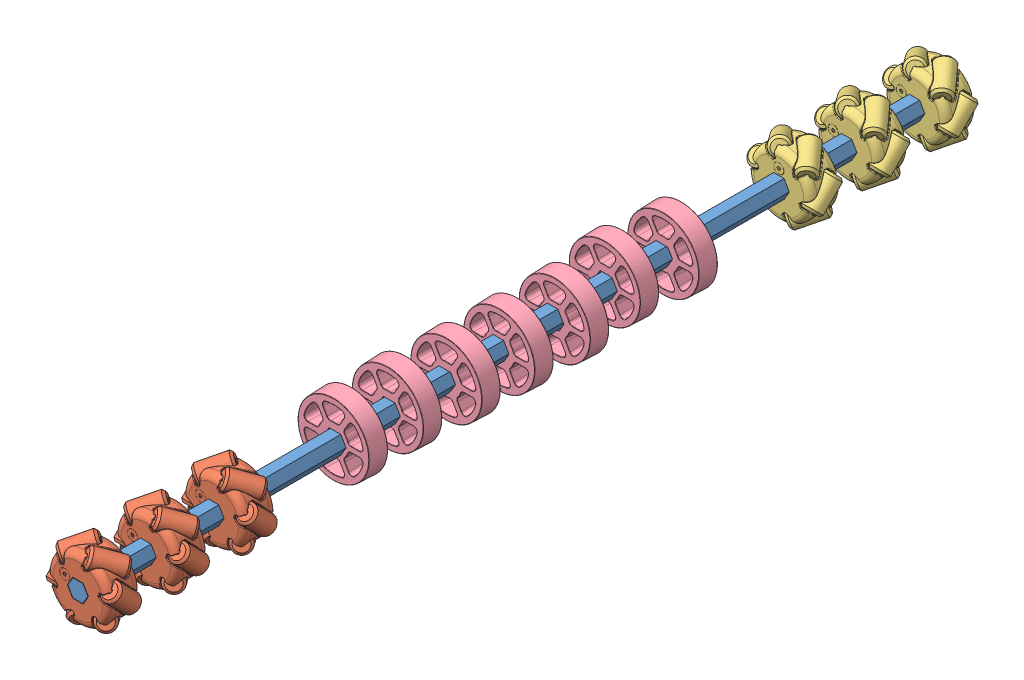
SolidWorks assembly mech intake, configuration Default. Lengths in mm.
Overall size (70.21 69.88 611.73).
14 component instances, 4 part files, 41 mates.
Components (placement in the parent):
- Hex shaft 0.5-1: Hex shaft 0.5 [Default] at (18.4614 91.3272 95.7371) size (14.66 12.7 609.6)
- TTB-0010-RH-1: TTB-0010-RH [Default] at (18.5054 91.3272 116.3746) x (-0.866025 0.5 0) z (0.5 0.866025 0) size (51.61 24.36 50.8)
- TTB-0010-RH-2: TTB-0010-RH [Default] at (18.5054 91.3272 163.9996) x (-0.866025 0.5 0) z (0.5 0.866025 0) size (51.61 24.36 50.8)
- TTB-0010-RH-3: TTB-0010-RH [Default] at (18.4834 91.3653 211.6246) x (-0.866025 0.5 0) z (0.5 0.866025 0) size (51.61 24.36 50.8)
- TTB-0010-LH-1: TTB-0010-LH [Default] at (18.5274 91.3653 -280.5004) x (0 -1 0) z (-1 0 0) size (51.61 24.36 50.8)
- TTB-0010-LH-2: TTB-0010-LH [Default] at (18.4834 91.3653 -375.7504) x (0.866025 -0.5 0) z (-0.5 -0.866025 0) size (51.61 24.36 50.8)
- TTB-0010-LH-3: TTB-0010-LH [Default] at (18.3954 91.2891 -328.1254) x (0.866025 -0.5 0) z (-0.5 -0.866025 0) size (51.61 24.36 50.8)
- 2in compliant wheel-1: 2in compliant wheel [Default] at (19.8179 90.3747 -123.3379) size (50.78 50.78 12.71)
- 2in compliant wheel-2: 2in compliant wheel [Default] at (19.9645 92.0257 -47.1379) size (50.78 50.78 12.71)
- 2in compliant wheel-3: 2in compliant wheel [Default] at (19.0113 90.3747 -85.2379) size (50.78 50.78 12.71)
- 2in compliant wheel-4: 2in compliant wheel [Default] at (16.9583 92.0257 29.0621) size (50.78 50.78 12.71)
- 2in compliant wheel-5: 2in compliant wheel [Default] at (19.9645 92.0257 -199.5379) size (50.78 50.78 12.71)
- 2in compliant wheel-7: 2in compliant wheel [Default] at (16.8116 92.2797 -161.4379) size (50.78 50.78 12.71)
- 2in compliant wheel-9: 2in compliant wheel [Default] at (16.9583 92.0257 -9.0379) size (50.78 50.78 12.71)
Mates (geometry in assembly coordinates):
- Coincident1: coincident anti-aligned: plane of Hex shaft 0.5-1 through (14.7952 97.6772 -386.8629) normal (-0.866025 0.5 0); plane of TTB-0010-RH-1 through (14.8172 97.7153 127.4871) normal (0.866025 -0.5 0)
- Coincident2: coincident anti-aligned: plane of Hex shaft 0.5-1 through (11.129 91.3272 -386.8629) normal (-0.866025 -0.5 0); plane of TTB-0010-RH-1 through (11.129 91.3272 127.4871) normal (0.866025 0.5 0)
- Coincident3: coincident anti-aligned: plane of Hex shaft 0.5-1 through (11.129 91.3272 -386.8629) normal (-0.866025 -0.5 0); plane of TTB-0010-RH-2 through (11.129 91.3272 175.1121) normal (0.866025 0.5 0)
- Coincident4: coincident anti-aligned: plane of Hex shaft 0.5-1 through (14.7952 97.6772 -386.8629) normal (-0.866025 0.5 0); plane of TTB-0010-RH-2 through (14.8172 97.7153 175.1121) normal (0.866025 -0.5 0)
- Coincident5: coincident anti-aligned: plane of Hex shaft 0.5-1 through (11.129 91.3272 -386.8629) normal (-0.866025 -0.5 0); plane of TTB-0010-RH-3 through (11.107 91.3653 222.7371) normal (0.866025 0.5 0)
- Coincident7: coincident anti-aligned: plane of Hex shaft 0.5-1 through (11.129 91.3272 -386.8629) normal (-0.866025 -0.5 0); plane of TTB-0010-RH-3 through (11.107 91.3653 222.7371) normal (0.866025 0.5 0)
- Coincident8: coincident anti-aligned: plane of Hex shaft 0.5-1 through (14.7952 84.9772 -386.8629) normal (0 -1 0); plane of TTB-0010-RH-3 through (14.7952 84.9772 222.7371) normal (0 1 0)
- Coincident9: coincident anti-aligned: plane of Hex shaft 0.5-1 through (14.7952 84.9772 -386.8629) normal (0 -1 0); plane of TTB-0010-LH-2 through (22.1716 84.9772 -364.6379) normal (0 1 0)
- Parallel1: parallel anti-aligned: plane of Hex shaft 0.5-1 through (22.1276 97.6772 -386.8629) normal (0 1 0); plane of TTB-0010-LH-2 through (14.7952 97.7534 -364.6379) normal (0 -1 0)
- Coincident11: coincident anti-aligned: plane of Hex shaft 0.5-1 through (11.129 91.3272 -386.8629) normal (-0.866025 -0.5 0); plane of TTB-0010-LH-2 through (14.7952 84.9772 -364.6379) normal (0.866025 0.5 0)
- Coincident12: coincident anti-aligned: plane of Hex shaft 0.5-1 through (14.7952 84.9772 -386.8629) normal (0 -1 0); plane of TTB-0010-LH-1 through (22.2156 84.9772 -269.3879) normal (0 1 0)
- Coincident13: coincident anti-aligned: plane of Hex shaft 0.5-1 through (14.7952 97.6772 -386.8629) normal (-0.866025 0.5 0); plane of TTB-0010-LH-1 through (11.151 91.3653 -269.3879) normal (0.866025 -0.5 0)
- Coincident15: coincident anti-aligned: plane of Hex shaft 0.5-1 through (22.1276 84.9772 -386.8629) normal (0.866025 -0.5 0); plane of TTB-0010-LH-3 through (25.7717 91.2891 -317.0129) normal (-0.866025 0.5 0)
- Coincident17: coincident anti-aligned: plane of Hex shaft 0.5-1 through (22.1276 97.6772 -386.8629) normal (0 1 0); plane of TTB-0010-LH-3 through (14.7072 97.6772 -317.0129) normal (0 -1 0)
- Coincident22: coincident aligned: plane of Hex shaft 0.5-1 through (18.4614 91.3272 -386.8629) normal (0 0 -1); plane of TTB-0010-LH-2 through (18.4834 91.3653 -386.8629) normal (0 0 -1)
- Distance2: distance = 25.4 mm anti-aligned: plane of TTB-0010-LH-2 through (18.4834 91.3653 -364.6379) normal (0 0 1); plane of TTB-0010-LH-3 through (18.3954 91.2891 -339.2379) normal (0 0 -1)
- Distance3: distance = 25.4 mm: plane of TTB-0010-LH-1 through (18.5274 91.3653 -291.6129) normal (0 0 -1); point of TTB-0010-LH-3
- Coincident29: coincident aligned: plane of Hex shaft 0.5-1 through (18.4614 91.3272 222.7371) normal (0 0 1); plane of TTB-0010-RH-3 through (18.4834 91.3653 222.7371) normal (0 0 1)
- Distance5: distance = 25.4 mm anti-aligned: plane of TTB-0010-RH-2 through (18.5054 91.3272 175.1121) normal (0 0 1); plane of TTB-0010-RH-3 through (18.4834 91.3653 200.5121) normal (0 0 -1)
- Distance6: distance = 25.4 mm anti-aligned: plane of TTB-0010-RH-2 through (18.5054 91.3272 152.8871) normal (0 0 -1); plane of TTB-0010-RH-1 through (18.5054 91.3272 127.4871) normal (0 0 1)
- Coincident32: coincident anti-aligned: plane of Hex shaft 0.5-1 through (22.1276 84.9772 -386.8629) normal (0.866025 -0.5 0); plane of 2in compliant wheel-2 through (26.197 92.0257 -34.436) normal (-0.866025 0.5 0)
- Coincident33: coincident: plane of Hex shaft 0.5-1 through (22.1276 97.6772 -386.8629) normal (0 1 0); line of 2in compliant wheel-2 through (23.2274 97.6772 -47.1379) axis (-1 0 0)
- Coincident34: coincident anti-aligned: plane of Hex shaft 0.5-1 through (14.7952 84.9772 -386.8629) normal (0 -1 0); plane of 2in compliant wheel-3 through (22.1276 84.9772 -72.536) normal (0 1 0)
- Parallel2: parallel anti-aligned: plane of Hex shaft 0.5-1 through (22.1276 97.6772 -386.8629) normal (0 1 0); plane of 2in compliant wheel-3 through (15.8951 95.7722 -72.536) normal (0 -1 0)
- Coincident36: coincident anti-aligned: plane of Hex shaft 0.5-1 through (22.1276 84.9772 -386.8629) normal (0.866025 -0.5 0); plane of 2in compliant wheel-3 through (25.2438 90.3747 -72.536) normal (-0.866025 0.5 0)
- Coincident37: coincident anti-aligned: plane of Hex shaft 0.5-1 through (22.1276 97.6772 -386.8629) normal (0 1 0); plane of 2in compliant wheel-7 through (13.6954 97.6772 -148.736) normal (0 -1 0)
- Coincident41: coincident: plane of Hex shaft 0.5-1 through (22.1276 97.6772 -386.8629) normal (0 1 0); line of 2in compliant wheel-9 through (20.2212 97.6772 -9.0379) axis (-1 0 0)
- Coincident42: coincident anti-aligned: plane of Hex shaft 0.5-1 through (11.129 91.3272 -386.8629) normal (-0.866025 -0.5 0); plane of 2in compliant wheel-9 through (13.842 86.6282 3.664) normal (0.866025 0.5 0)
- Coincident43: coincident: plane of Hex shaft 0.5-1 through (22.1276 97.6772 -386.8629) normal (0 1 0); line of 2in compliant wheel-4 through (20.2212 97.6772 29.0621) axis (-1 0 0)
- Coincident44: coincident anti-aligned: plane of Hex shaft 0.5-1 through (11.129 91.3272 -386.8629) normal (-0.866025 -0.5 0); plane of 2in compliant wheel-4 through (13.842 86.6282 41.764) normal (0.866025 0.5 0)
- Distance9: distance = 25.4 mm anti-aligned: plane of 2in compliant wheel-4 through (16.9583 92.0257 29.0621) normal (0 0 -1); plane of 2in compliant wheel-9 through (16.9583 92.0257 3.6621) normal (0 0 1)
- Distance10: distance = 25.4 mm anti-aligned: plane of 2in compliant wheel-2 through (19.9645 92.0257 -34.4379) normal (0 0 1); plane of 2in compliant wheel-9 through (16.9583 92.0257 -9.0379) normal (0 0 -1)
- Distance11: distance = 25.4 mm anti-aligned: plane of 2in compliant wheel-3 through (19.0113 90.3747 -72.5379) normal (0 0 1); plane of 2in compliant wheel-2 through (19.9645 92.0257 -47.1379) normal (0 0 -1)
- Coincident50: coincident anti-aligned: plane of Hex shaft 0.5-1 through (14.7952 84.9772 -386.8629) normal (0 -1 0); plane of 2in compliant wheel-1 through (22.9341 84.9772 -110.636) normal (0 1 0)
- Coincident52: coincident: plane of Hex shaft 0.5-1 through (25.7937 91.3272 -386.8629) normal (0.866025 0.5 0); line of 2in compliant wheel-1 through (23.0808 96.0262 -110.6379) axis (0.5 -0.866025 0)
- Distance12: distance = 25.4 mm anti-aligned: plane of 2in compliant wheel-1 through (19.8179 90.3747 -110.6379) normal (0 0 1); plane of 2in compliant wheel-3 through (19.0113 90.3747 -85.2379) normal (0 0 -1)
- Coincident55: coincident: plane of Hex shaft 0.5-1 through (22.1276 97.6772 -386.8629) normal (0 1 0); line of 2in compliant wheel-5 through (16.7016 97.6772 -186.8379) axis (1 0 0)
- Coincident56: coincident anti-aligned: plane of Hex shaft 0.5-1 through (22.1276 84.9772 -386.8629) normal (0.866025 -0.5 0); plane of 2in compliant wheel-5 through (26.197 92.0257 -186.836) normal (-0.866025 0.5 0)
- Distance13: distance = 25.4 mm anti-aligned: plane of 2in compliant wheel-5 through (19.9645 92.0257 -186.8379) normal (0 0 1); plane of 2in compliant wheel-7 through (16.8116 92.2797 -161.4379) normal (0 0 -1)
- Distance14: distance = 25.4 mm anti-aligned: plane of 2in compliant wheel-7 through (16.8116 92.2797 -148.7379) normal (0 0 1); plane of 2in compliant wheel-1 through (19.8179 90.3747 -123.3379) normal (0 0 -1)
- Coincident59: coincident anti-aligned: plane of Hex shaft 0.5-1 through (11.129 91.3272 -386.8629) normal (-0.866025 -0.5 0); plane of 2in compliant wheel-7 through (13.6954 86.8822 -148.736) normal (0.866025 0.5 0)
